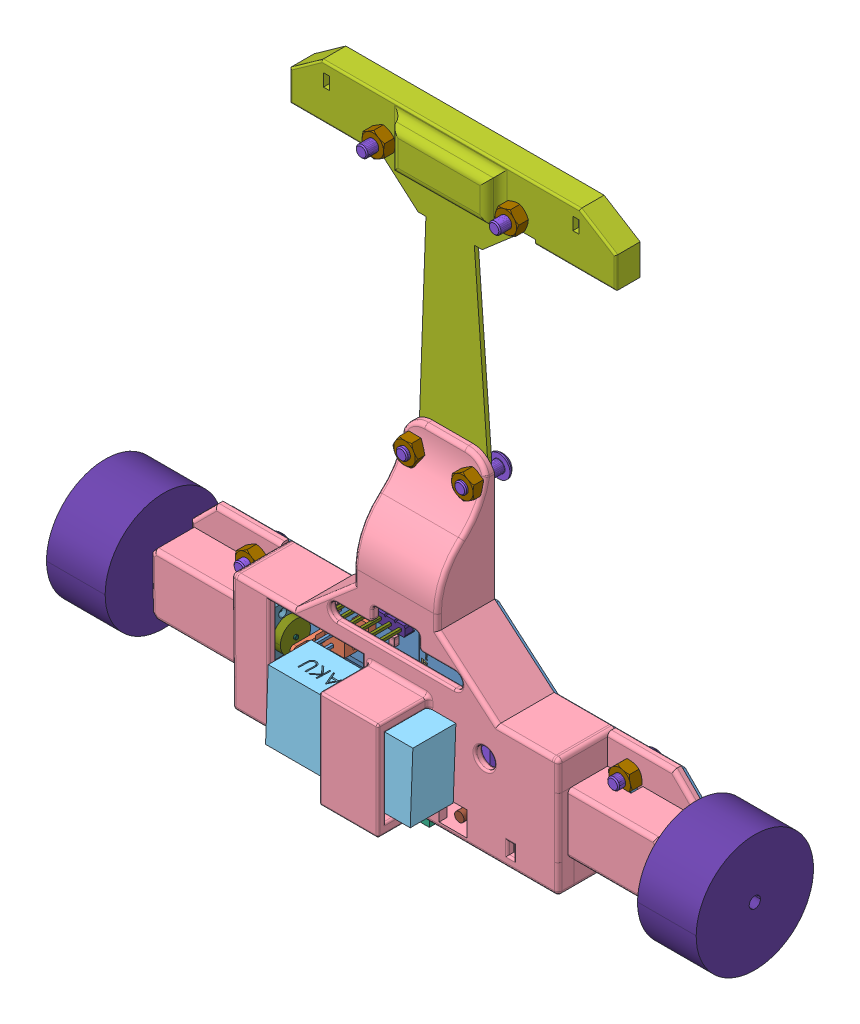
SolidWorks assembly LF_v5_TotalComplexOfRobot, configuration Domyślna. Lengths in mm.
Overall size (166.18 143.38 42.71).
437 component instances, 57 part files, 36 mates.
Components (placement in the parent):
- LF_v5_LowerPartOfHousing-1: LF_v5_LowerPartOfHousing [Domyślna] at (-21.7771 -53.6224 135.3929) size (130 132.75 5.29) (hidden)
- LF_v5_BoardWithSensors.STEP-1: LF_v5_BoardWithSensors.STEP [Domyślna] at (-37.5021 69.0607 133.6929) size (81 20.29 4.87) (hidden)
  - LFEK_Czujniki_v4P_G.step.STEP-1: LFEK_Czujniki_v4P_G.step.STEP [Domyślna] at origin size (81 20.29 4.87)
    - BoardCZV.step.STEP-1: BoardCZV.step.STEP [Domyślna] at origin size (81 20.29 1.59)
      - Open CASCADE STEP translator 6.8 1.1.1.step.STEP-1: Open CASCADE STEP translator 6.8 1.1.1.step.STEP [Domyślna] at (0 0 -1.5914) size (81 20.29 1.59)
    - U8CZV.step.STEP-1: U8CZV.step.STEP [Domyślna] at origin size (4.19 3.05 2)
      - 6801970560.step.STEP-1: 6801970560.step.STEP [Domyślna] at (15.1904 6.573 -3.5914) size (4.19 3.05 2)
        - Extruded.step.STEP-1: Extruded.step.STEP [Domyślna] at origin size (4.19 3.05 2)
    - U7CZV.step.STEP-1: U7CZV.step.STEP [Domyślna] at origin size (4.19 3.05 2)
      - 6801970560.step.STEP-1: 6801970560.step.STEP [Domyślna] at (5.6904 2.473 -3.5914) size (4.19 3.05 2)
        - Extruded.step.STEP-1: Extruded.step.STEP [Domyślna] at origin size (4.19 3.05 2)
    - U6CZV.step.STEP-1: U6CZV.step.STEP [Domyślna] at origin size (4.19 3.05 2)
      - 6801970560.step.STEP-1: 6801970560.step.STEP [Domyślna] at (25.2904 6.673 -3.5914) size (4.19 3.05 2)
        - Extruded.step.STEP-1: Extruded.step.STEP [Domyślna] at origin size (4.19 3.05 2)
    - U5CZV.step.STEP-1: U5CZV.step.STEP [Domyślna] at origin size (4.19 3.05 2)
      - 6801970560.step.STEP-1: 6801970560.step.STEP [Domyślna] at (34.9905 6.673 -3.5914) size (4.19 3.05 2)
        - Extruded.step.STEP-1: Extruded.step.STEP [Domyślna] at origin size (4.19 3.05 2)
    - U4CZV.step.STEP-1: U4CZV.step.STEP [Domyślna] at origin size (4.19 3.05 2)
      - 6801970560.step.STEP-1: 6801970560.step.STEP [Domyślna] at (44.9905 6.673 -3.5914) size (4.19 3.05 2)
        - Extruded.step.STEP-1: Extruded.step.STEP [Domyślna] at origin size (4.19 3.05 2)
    - U3CZV.step.STEP-1: U3CZV.step.STEP [Domyślna] at origin size (4.19 3.05 2)
      - 6801970560.step.STEP-1: 6801970560.step.STEP [Domyślna] at (54.9905 6.673 -3.5914) size (4.19 3.05 2)
        - Extruded.step.STEP-1: Extruded.step.STEP [Domyślna] at origin size (4.19 3.05 2)
    - U2CZV.step.STEP-1: U2CZV.step.STEP [Domyślna] at origin size (4.19 3.05 2)
      - 6801970560.step.STEP-1: 6801970560.step.STEP [Domyślna] at (64.9904 6.673 -3.5914) size (4.19 3.05 2)
        - Extruded.step.STEP-1: Extruded.step.STEP [Domyślna] at origin size (4.19 3.05 2)
    - U1CZV.step.STEP-1: U1CZV.step.STEP [Domyślna] at origin size (4.19 3.05 2)
      - 6801970560.step.STEP-1: 6801970560.step.STEP [Domyślna] at (74.7905 2.373 -3.5914) size (4.19 3.05 2)
        - Extruded.step.STEP-1: Extruded.step.STEP [Domyślna] at origin size (4.19 3.05 2)
    - D2CZV.step.STEP-1: D2CZV.step.STEP [Domyślna] at origin size (1.6 3.2 1.1)
      - D1206_2.step.STEP-1: D1206_2.step.STEP [Domyślna] at (8.2001 8.2337 0.2489) x (0 1 0) z (1 0 0) size (3.2 1.1 1.6)
    - D1CZV.step.STEP-1: D1CZV.step.STEP [Domyślna] at origin size (1.6 3.2 1.1)
      - D1206_2.step.STEP-1: D1206_2.step.STEP [Domyślna] at (71.9999 8.3333 0.2489) x (0 -1 0) z (-1 0 0) size (3.2 1.1 1.6)
    - J1CZV.step.STEP-1: J1CZV.step.STEP [Domyślna] at origin size (15.7 4.25 1.29)
      - 687120183722.step.STEP-1: 687120183722.step.STEP [Domyślna] at (39.9501 4.8501 0.64) x (1 0 0) z (0 0 1) size (15.7 4.25 1.29)
        - 68x120183x22.step.STEP-1: 68x120183x22.step.STEP [Domyślna] at origin size (13 3.1 1.2)
        - 68X1xx183x22_Pin_Bottom.step.STEP-1: 68X1xx183x22_Pin_Bottom.step.STEP [Domyślna] at (-4.65 1.05 0.005) x (0 1 0) z (0 0 1) size (3.1 0.2 1.15)
        - 68x120183x22_Actuator.step.STEP-1: 68x120183x22_Actuator.step.STEP [Domyślna] at (0 -2 0) x (1 0 0) z (0 0 -1) size (15.7 3.8 1.1)
        - 68X1XX183X22_Solder_Pad.step.STEP-1: 68X1XX183X22_Solder_Pad.step.STEP [Domyślna] at (5.55 -0.25 0.02) x (0 -1 0) z (0 0 1) size (2.5 2 1.24)
        - 68X1xx183x22_Solder_Pad2.step.STEP-1: 68X1xx183x22_Solder_Pad2.step.STEP [Domyślna] at (-5.55 -0.25 0.02) x (0 -1 0) z (0 0 -1) size (2.5 2 1.24)
        - 68X1xx183x22_Pin_Bottom.step.STEP-2: 68X1xx183x22_Pin_Bottom.step.STEP [Domyślna] at (-4.15 1.05 0.005) x (0 1 0) z (0 0 1) size (3.1 0.2 1.15)
        - 68X1xx183x22_Pin_Bottom.step.STEP-3: 68X1xx183x22_Pin_Bottom.step.STEP [Domyślna] at (-3.65 1.05 0.005) x (0 1 0) z (0 0 1) size (3.1 0.2 1.15)
        - 68X1xx183x22_Pin_Bottom.step.STEP-4: 68X1xx183x22_Pin_Bottom.step.STEP [Domyślna] at (-3.15 1.05 0.005) x (0 1 0) z (0 0 1) size (3.1 0.2 1.15)
        - 68X1xx183x22_Pin_Bottom.step.STEP-5: 68X1xx183x22_Pin_Bottom.step.STEP [Domyślna] at (-2.65 1.05 0.005) x (0 1 0) z (0 0 1) size (3.1 0.2 1.15)
        - 68X1xx183x22_Pin_Bottom.step.STEP-6: 68X1xx183x22_Pin_Bottom.step.STEP [Domyślna] at (-2.15 1.05 0.005) x (0 1 0) z (0 0 1) size (3.1 0.2 1.15)
        - 68X1xx183x22_Pin_Bottom.step.STEP-7: 68X1xx183x22_Pin_Bottom.step.STEP [Domyślna] at (-1.65 1.05 0.005) x (0 1 0) z (0 0 1) size (3.1 0.2 1.15)
        - 68X1xx183x22_Pin_Bottom.step.STEP-8: 68X1xx183x22_Pin_Bottom.step.STEP [Domyślna] at (-1.15 1.05 0.005) x (0 1 0) z (0 0 1) size (3.1 0.2 1.15)
        - 68X1xx183x22_Pin_Bottom.step.STEP-9: 68X1xx183x22_Pin_Bottom.step.STEP [Domyślna] at (-0.65 1.05 0.005) x (0 1 0) z (0 0 1) size (3.1 0.2 1.15)
        - 68X1xx183x22_Pin_Bottom.step.STEP-10: 68X1xx183x22_Pin_Bottom.step.STEP [Domyślna] at (-0.15 1.05 0.005) x (0 1 0) z (0 0 1) size (3.1 0.2 1.15)
        - 68X1xx183x22_Pin_Bottom.step.STEP-11: 68X1xx183x22_Pin_Bottom.step.STEP [Domyślna] at (0.35 1.05 0.005) x (0 1 0) z (0 0 1) size (3.1 0.2 1.15)
        - 68X1xx183x22_Pin_Bottom.step.STEP-12: 68X1xx183x22_Pin_Bottom.step.STEP [Domyślna] at (0.85 1.05 0.005) x (0 1 0) z (0 0 1) size (3.1 0.2 1.15)
        - 68X1xx183x22_Pin_Bottom.step.STEP-13: 68X1xx183x22_Pin_Bottom.step.STEP [Domyślna] at (1.35 1.05 0.005) x (0 1 0) z (0 0 1) size (3.1 0.2 1.15)
        - 68X1xx183x22_Pin_Bottom.step.STEP-14: 68X1xx183x22_Pin_Bottom.step.STEP [Domyślna] at (1.85 1.05 0.005) x (0 1 0) z (0 0 1) size (3.1 0.2 1.15)
        - 68X1xx183x22_Pin_Bottom.step.STEP-15: 68X1xx183x22_Pin_Bottom.step.STEP [Domyślna] at (2.35 1.05 0.005) x (0 1 0) z (0 0 1) size (3.1 0.2 1.15)
        - 68X1xx183x22_Pin_Bottom.step.STEP-16: 68X1xx183x22_Pin_Bottom.step.STEP [Domyślna] at (2.85 1.05 0.005) x (0 1 0) z (0 0 1) size (3.1 0.2 1.15)
        - 68X1xx183x22_Pin_Bottom.step.STEP-17: 68X1xx183x22_Pin_Bottom.step.STEP [Domyślna] at (3.35 1.05 0.005) x (0 1 0) z (0 0 1) size (3.1 0.2 1.15)
        - 68X1xx183x22_Pin_Bottom.step.STEP-18: 68X1xx183x22_Pin_Bottom.step.STEP [Domyślna] at (3.85 1.05 0.005) x (0 1 0) z (0 0 1) size (3.1 0.2 1.15)
        - 68X1xx183x22_Pin_Bottom.step.STEP-19: 68X1xx183x22_Pin_Bottom.step.STEP [Domyślna] at (4.35 1.05 0.005) x (0 1 0) z (0 0 1) size (3.1 0.2 1.15)
        - 68X1xx183x22_Pin_Bottom.step.STEP-20: 68X1xx183x22_Pin_Bottom.step.STEP [Domyślna] at (4.85 1.05 0.005) x (0 1 0) z (0 0 1) size (3.1 0.2 1.15)
    - R1CZV.step.STEP-1: R1CZV.step.STEP [Domyślna] at origin size (1.25 2 0.6)
      - User_Library-SMD_RESISTOR-10805.step.STEP-1: User_Library-SMD_RESISTOR-10805.step.STEP [Domyślna] at (78.94 2.4538 -1.881) x (1 0 0) z (0 -1 0) size (1.25 0.6 2)
    - R2CZV.step.STEP-1: R2CZV.step.STEP [Domyślna] at origin size (1.25 2 0.6)
      - User_Library-SMD_RESISTOR-10805.step.STEP-1: User_Library-SMD_RESISTOR-10805.step.STEP [Domyślna] at (59.1239 6.7758 -1.881) x (1 0 0) z (0 -1 0) size (1.25 0.6 2)
    - R3CZV.step.STEP-1: R3CZV.step.STEP [Domyślna] at origin size (1.25 2 0.6)
      - User_Library-SMD_RESISTOR-10805.step.STEP-1: User_Library-SMD_RESISTOR-10805.step.STEP [Domyślna] at (48.7205 6.6898 -1.881) x (1 0 0) z (0 -1 0) size (1.25 0.6 2)
    - R4CZV.step.STEP-1: R4CZV.step.STEP [Domyślna] at origin size (1.25 2 0.6)
      - User_Library-SMD_RESISTOR-10805.step.STEP-1: User_Library-SMD_RESISTOR-10805.step.STEP [Domyślna] at (68.9209 6.8237 -1.881) x (1 0 0) z (0 -1 0) size (1.25 0.6 2)
    - R5CZV.step.STEP-1: R5CZV.step.STEP [Domyślna] at origin size (2 1.25 0.6)
      - User_Library-SMD_RESISTOR-10805.step.STEP-1: User_Library-SMD_RESISTOR-10805.step.STEP [Domyślna] at (69.9592 3.2749 -1.881) x (0 1 0) z (1 0 0) size (1.25 0.6 2)
    - R6CZV.step.STEP-1: R6CZV.step.STEP [Domyślna] at origin size (1.25 2 0.6)
      - User_Library-SMD_RESISTOR-10805.step.STEP-1: User_Library-SMD_RESISTOR-10805.step.STEP [Domyślna] at (50.6149 6.6488 -1.881) x (1 0 0) z (0 -1 0) size (1.25 0.6 2)
    - R7CZV.step.STEP-1: R7CZV.step.STEP [Domyślna] at origin size (2 1.25 0.6)
      - User_Library-SMD_RESISTOR-10805.step.STEP-1: User_Library-SMD_RESISTOR-10805.step.STEP [Domyślna] at (45.1658 9.5901 -1.881) x (0 -1 0) z (-1 0 0) size (1.25 0.6 2)
    - R8CZV.step.STEP-1: R8CZV.step.STEP [Domyślna] at origin size (1.25 2 0.6)
      - User_Library-SMD_RESISTOR-10805.step.STEP-1: User_Library-SMD_RESISTOR-10805.step.STEP [Domyślna] at (61.1499 6.7158 -1.881) x (1 0 0) z (0 -1 0) size (1.25 0.6 2)
    - R9CZV.step.STEP-1: R9CZV.step.STEP [Domyślna] at origin size (2 1.25 0.6)
      - User_Library-SMD_RESISTOR-10805.step.STEP-1: User_Library-SMD_RESISTOR-10805.step.STEP [Domyślna] at (34.7912 9.608 -1.881) x (0 1 0) z (1 0 0) size (1.25 0.6 2)
    - R10CZV.step.STEP-1: R10CZV.step.STEP [Domyślna] at origin size (1.25 2 0.6)
      - User_Library-SMD_RESISTOR-10805.step.STEP-1: User_Library-SMD_RESISTOR-10805.step.STEP [Domyślna] at (29.0439 6.7928 -1.881) x (1 0 0) z (0 -1 0) size (1.25 0.6 2)
    - R11CZV.step.STEP-1: R11CZV.step.STEP [Domyślna] at origin size (2 1.25 0.6)
      - User_Library-SMD_RESISTOR-10805.step.STEP-1: User_Library-SMD_RESISTOR-10805.step.STEP [Domyślna] at (7.9162 5.5999 -1.881) x (0 1 0) z (1 0 0) size (1.25 0.6 2)
    - R12CZV.step.STEP-1: R12CZV.step.STEP [Domyślna] at origin size (1.25 2 0.6)
      - User_Library-SMD_RESISTOR-10805.step.STEP-1: User_Library-SMD_RESISTOR-10805.step.STEP [Domyślna] at (19.1249 6.6337 -1.881) x (1 0 0) z (0 -1 0) size (1.25 0.6 2)
    - R13CZV.step.STEP-1: R13CZV.step.STEP [Domyślna] at origin size (1.25 2 0.6)
      - User_Library-SMD_RESISTOR-10805.step.STEP-1: User_Library-SMD_RESISTOR-10805.step.STEP [Domyślna] at (31.0839 6.9058 -1.881) x (1 0 0) z (0 -1 0) size (1.25 0.6 2)
    - R14CZV.step.STEP-1: R14CZV.step.STEP [Domyślna] at origin size (1.25 2 0.6)
      - User_Library-SMD_RESISTOR-10805.step.STEP-1: User_Library-SMD_RESISTOR-10805.step.STEP [Domyślna] at (21.3409 6.6698 -1.881) x (1 0 0) z (0 -1 0) size (1.25 0.6 2)
    - R15CZV.step.STEP-1: R15CZV.step.STEP [Domyślna] at origin size (1.25 2 0.6)
      - User_Library-SMD_RESISTOR-10805.step.STEP-1: User_Library-SMD_RESISTOR-10805.step.STEP [Domyślna] at (11.3899 6.7318 -1.881) x (1 0 0) z (0 -1 0) size (1.25 0.6 2)
    - R16CZV.step.STEP-1: R16CZV.step.STEP [Domyślna] at origin size (1.25 2 0.6)
      - User_Library-SMD_RESISTOR-10805.step.STEP-1: User_Library-SMD_RESISTOR-10805.step.STEP [Domyślna] at (1.6869 2.2537 -1.881) x (1 0 0) z (0 -1 0) size (1.25 0.6 2)
- LF_v5_MainElectricalBoardwithMCU.step-1: LF_v5_MainElectricalBoardwithMCU.step [Domyślna] at (-21.7771 -53.6224 135.3929) size (166.18 41.84 30.14)
  - BoardFF.step-1: BoardFF.step [Domyślna] at origin size (130 40.35 1.59)
    - Open CASCADE STEP translator 6.8 2.1.1.step-1: Open CASCADE STEP translator 6.8 2.1.1.step [Domyślna] at (0 0 -1.5914) size (130 40.35 1.59)
  - CMJ1FF.step-1: CMJ1FF.step [Domyślna] at origin size (4.19 3.05 2)
    - 6480266160.step-1: 6480266160.step [Domyślna] at (3.27 16.79 0) size (4.19 3.05 2)
      - Extruded.step-1: Extruded.step [Domyślna] at origin size (4.19 3.05 2)
  - CMJ2FF.step-1: CMJ2FF.step [Domyślna] at origin size (8.61 4.54 5)
    - 6480265920.step-1: 6480265920.step [Domyślna] at (47.73 6.385 0) size (8.61 4.54 5)
      - Extruded-0.step-1: Extruded-0.step [Domyślna] at origin size (8.61 4.54 5)
  - C4FF.step-1: C4FF.step [Domyślna] at origin size (1.35 2.1 1.35)
    - 0805C.step-1: 0805C.step [Domyślna] at (54.4661 6.0661 0) x (0 -1 0) z (0 0 1) size (2.1 1.35 1.35)
      - Open CASCADE STEP translator 6.8 2.4.1.1.step-1: Open CASCADE STEP translator 6.8 2.4.1.1.step [Domyślna] at origin size (2.1 1.35 1.35)
      - Open CASCADE STEP translator 6.8 2.4.1.2.step-1: Open CASCADE STEP translator 6.8 2.4.1.2.step [Domyślna] at origin
  - U6FF.step-1: U6FF.step [Domyślna] at origin size (7 6.5 1.65)
    - SOT-223.step-1: SOT-223.step [Domyślna] at (3.0406 1.7749 -2.3167) x (-1 0 0) z (0 -1 0) size (7 1.65 6.5)
  - 16FF.step-1: 16FF.step [Domyślna] at origin size (3.39 1.6 1.65)
    - 3216-SMDA.step-1: 3216-SMDA.step [Domyślna] at (47.0511 -1.8714 -0.4115) x (1 0 0) z (0 0 1) size (3.39 1.6 1.65)
      - User_Library-Tantalum_Capacitor_Case_A_Tantalum_case_A_part1.step-1: User_Library-Tantalum_Capacitor_Case_A_Tantalum_case_A_part1.step [Domyślna] at (-1.4503 0.3155 0.551) size (3.2 1.6 1.6)
      - User_Library-Tantalum_Capacitor_Case_A_Tantalum_case_A_part2.step-1: User_Library-Tantalum_Capacitor_Case_A_Tantalum_case_A_part2.step [Domyślna] at (-0.7455 0.5155 0.501) x (-1 0 0) z (0 0 -1) size (0.8 1.2 0.9)
      - User_Library-Tantalum_Capacitor_Case_A_Tantalum_case_A_part2.step-2: User_Library-Tantalum_Capacitor_Case_A_Tantalum_case_A_part2.step [Domyślna] at (1.0449 1.7155 0.501) x (1 0 0) z (0 0 -1) size (0.8 1.2 0.9)
  - D4FF.step-1: D4FF.step [Domyślna] at origin size (6.11 8.13 2.39)
    - DO214AB.step-1: DO214AB.step [Domyślna] at (-8.5231 8.9094 -1.566) x (0 1 0) z (0 0 -1) size (8.13 6.11 2.39)
  - P3FF.step-1: P3FF.step [Domyślna] at origin size (2.54 10.16 11.54)
    - 61300411121.step-1: 61300411121.step [Domyślna] at (13.85 2.18 1.3) x (0 1 0) z (1 0 0) size (10.16 11.54 2.54)
      - 6130xx11121_PIN.step-1: 6130xx11121_PIN.step [Domyślna] at (-3.81 1.5 0) x (1 0 0) z (0 -1 0) size (0.64 0.64 11.54)
      - 6130xx11121_PIN.step-2: 6130xx11121_PIN.step [Domyślna] at (-1.27 1.5 0) x (1 0 0) z (0 -1 0) size (0.64 0.64 11.54)
      - 6130xx11121_PIN.step-3: 6130xx11121_PIN.step [Domyślna] at (1.27 1.5 0) x (1 0 0) z (0 -1 0) size (0.64 0.64 11.54)
      - 6130xx11121_PIN.step-4: 6130xx11121_PIN.step [Domyślna] at (3.81 1.5 0) x (1 0 0) z (0 -1 0) size (0.64 0.64 11.54)
      - 61300411121-1.step-1: 61300411121-1.step [Domyślna] at origin size (10.16 2.54 2.54)
  - IR_TSOP2236FF.step-1: IR_TSOP2236FF.step [Domyślna] at origin size (2.4 2.4 13)
    - 6479903328.step-1: 6479903328.step [Domyślna] at (39.625 -1.7875 0) x (-1 0 0) z (0 0 1) size (2.4 2.4 13)
      - Cylinder.step-1: Cylinder.step [Domyślna] at origin size (2.4 2.4 13)
  - R10FF.step-1: R10FF.step [Domyślna] at origin size (2 1.25 0.6)
    - User_Library-SMD_RESISTOR-10805.step-1: User_Library-SMD_RESISTOR-10805.step [Domyślna] at (14.3657 29.675 0.2896) x (0 -1 0) z (-1 0 0) size (1.25 0.6 2)
  - R9FF.step-1: R9FF.step [Domyślna] at origin size (2 1.25 0.6)
    - User_Library-SMD_RESISTOR-10805.step-1: User_Library-SMD_RESISTOR-10805.step [Domyślna] at (14.3907 31.6001 0.2896) x (0 -1 0) z (-1 0 0) size (1.25 0.6 2)
  - C25FF.step-1: C25FF.step [Domyślna] at origin size (1.35 2.1 1.35)
    - 0805C.step-1: 0805C.step [Domyślna] at (43.9001 15.4161 0) x (0 -1 0) z (0 0 1) size (2.1 1.35 1.35)
      - Open CASCADE STEP translator 6.8 2.4.1.1.step-1: Open CASCADE STEP translator 6.8 2.4.1.1.step [Domyślna] at origin size (2.1 1.35 1.35)
      - Open CASCADE STEP translator 6.8 2.4.1.2.step-1: Open CASCADE STEP translator 6.8 2.4.1.2.step [Domyślna] at origin
  - C30FF.step-1: C30FF.step [Domyślna] at origin size (1.35 2.1 1.35)
    - 0805C.step-1: 0805C.step [Domyślna] at (43.8749 17.3089 0) x (0 1 0) z (0 0 1) size (2.1 1.35 1.35)
      - Open CASCADE STEP translator 6.8 2.4.1.1.step-1: Open CASCADE STEP translator 6.8 2.4.1.1.step [Domyślna] at origin size (2.1 1.35 1.35)
      - Open CASCADE STEP translator 6.8 2.4.1.2.step-1: Open CASCADE STEP translator 6.8 2.4.1.2.step [Domyślna] at origin
  - C28FF.step-1: C28FF.step [Domyślna] at origin size (1.71 3.2 1.71)
    - User_Library-Capacitor_Vishay_1206_X7R.step-1: User_Library-Capacitor_Vishay_1206_X7R.step [Domyślna] at (14.9319 10.1506 -0.0102) x (0 1 0) z (0 0 1) size (3.2 1.7 1.7)
  - R14FF.step-1: R14FF.step [Domyślna] at origin size (1.25 2 0.6)
    - User_Library-SMD_RESISTOR-10805.step-1: User_Library-SMD_RESISTOR-10805.step [Domyślna] at (41.1749 1.7657 0.2896) x (1 0 0) z (0 -1 0) size (1.25 0.6 2)
  - R13FF.step-1: R13FF.step [Domyślna] at origin size (2 1.25 0.6)
    - User_Library-SMD_RESISTOR-10805.step-1: User_Library-SMD_RESISTOR-10805.step [Domyślna] at (37.4236 9.82 0.2896) x (0 -1 0) z (-1 0 0) size (1.25 0.6 2)
  - U2FF.step-1: U2FF.step [Domyślna] at origin size (49.09 30.14 30.14)
    - Silnik_enkAP214.step-1: Silnik_enkAP214.step [Domyślna] at (64.0421 1.0451 0) x (0 0 -1) z (0 1 0) size (30.14 49.09 30.14)
      - Enkoder_PCB.step-1: Enkoder_PCB.step [Domyślna] at (-5.6332 0.2835 8.6889) x (0 0 1) z (0 1 0) size (11.6 9.6 1.3)
      - micro-metal-gearmotor-backshaft.step.step-1: micro-metal-gearmotor-backshaft.step.step [Domyślna] at (-5.6332 -15.9165 8.6889) x (0 0 1) z (0 -1 0) size (12 10.04 40.2)
      - Dysk_pololu.step-1: Dysk_pololu.step [Domyślna] at (-5.6332 -14.4184 8.6889) x (0.89461 0 0.446849) z (0 1 0) size (7.7 7.7 2)
      - Dysk_pololu.step-2: Dysk_pololu.step [Domyślna] at (-5.6332 4.8635 8.6889) x (0.999981 0 -0.006181) z (0 -1 0) size (7.7 7.7 2)
      - Kolko.step-1: Kolko.step [Domyślna] at (-5.6332 -28.8098 8.6889) x (0.999989 0 -0.004766) z (0 -1 0) size (30 30 15)
  - U1FF.step-1: U1FF.step [Domyślna] at origin size (49.09 30.14 30.14)
    - Silnik_enkAP214.step-1: Silnik_enkAP214.step [Domyślna] at (-14.5171 18.505 0) x (0 0 -1) z (0 -1 0) size (30.14 49.09 30.14)
      - Enkoder_PCB.step-1: Enkoder_PCB.step [Domyślna] at (-5.6332 0.2835 8.6889) x (0 0 1) z (0 1 0) size (11.6 9.6 1.3)
      - micro-metal-gearmotor-backshaft.step.step-1: micro-metal-gearmotor-backshaft.step.step [Domyślna] at (-5.6332 -15.9165 8.6889) x (0 0 1) z (0 -1 0) size (12 10.04 40.2)
      - Dysk_pololu.step-1: Dysk_pololu.step [Domyślna] at (-5.6332 -14.4184 8.6889) x (0.89461 0 0.446849) z (0 1 0) size (7.7 7.7 2)
      - Dysk_pololu.step-2: Dysk_pololu.step [Domyślna] at (-5.6332 4.8635 8.6889) x (0.999981 0 -0.006181) z (0 -1 0) size (7.7 7.7 2)
      - Kolko.step-1: Kolko.step [Domyślna] at (-5.6332 -28.8098 8.6889) x (0.999989 0 -0.004766) z (0 -1 0) size (30 30 15)
  - Y1FF.step-1: Y1FF.step [Domyślna] at origin size (3.27 5.5 1.5)
    - 6479903888.step-1: 6479903888.step [Domyślna] at (41.0546 16.3547 0) size (3.27 5.5 1.5)
      - Extruded-2.step-1: Extruded-2.step [Domyślna] at origin size (3.27 5.5 1.5)
  - VIN_CONNECTOR1FF.step-1: VIN_CONNECTOR1FF.step [Domyślna] at origin size (5.8 5.08 14.9)
    - 61900211121.step-1: 61900211121.step [Domyślna] at (-2.2999 11.5249 5.78) x (0 1 0) z (0 0 1) size (5.08 5.8 14.9)
      - 6190xx11121_PIN.step-1: 6190xx11121_PIN.step [Domyślna] at (-1.27 0.3 -2.05) size (0.64 0.64 14.2)
      - 6190xx11121_PIN.step-2: 6190xx11121_PIN.step [Domyślna] at (1.27 0.3 -1.75) size (0.64 0.64 14.2)
      - 61900211121-3.step-1: 61900211121-3.step [Domyślna] at origin size (5.08 5.8 11.5)
  - U4FF.step-1: U4FF.step [Domyślna] at origin size (6.42 5 1)
    - PW0016AakaMTC16.step-1: PW0016AakaMTC16.step [Domyślna] at (47.7419 6.5511 -2.1914) x (0 -1 0) z (1 0 0) size (5 1 6.42)
      - BODY_MTC16.step-1: BODY_MTC16.step [Domyślna] at origin size (5 0.9 4.4)
      - LEAD_MTC16.step-1: LEAD_MTC16.step [Domyślna] at (2.275 -0.3725 -2.6) x (-1 0 0) z (0 0 -1) size (0.24 0.62 1.01)
      - LEAD_MTC16.step-2: LEAD_MTC16.step [Domyślna] at (1.625 -0.3725 -2.6) x (-1 0 0) z (0 0 -1) size (0.24 0.62 1.01)
      - LEAD_MTC16.step-3: LEAD_MTC16.step [Domyślna] at (0.975 -0.3725 -2.6) x (-1 0 0) z (0 0 -1) size (0.24 0.62 1.01)
      - LEAD_MTC16.step-4: LEAD_MTC16.step [Domyślna] at (0.325 -0.3725 -2.6) x (-1 0 0) z (0 0 -1) size (0.24 0.62 1.01)
      - LEAD_MTC16.step-5: LEAD_MTC16.step [Domyślna] at (-0.325 -0.3725 -2.6) x (-1 0 0) z (0 0 -1) size (0.24 0.62 1.01)
      - LEAD_MTC16.step-6: LEAD_MTC16.step [Domyślna] at (-0.975 -0.3725 -2.6) x (-1 0 0) z (0 0 -1) size (0.24 0.62 1.01)
      - LEAD_MTC16.step-7: LEAD_MTC16.step [Domyślna] at (-1.625 -0.3725 -2.6) x (-1 0 0) z (0 0 -1) size (0.24 0.62 1.01)
      - LEAD_MTC16.step-8: LEAD_MTC16.step [Domyślna] at (-2.275 -0.3725 -2.6) x (-1 0 0) z (0 0 -1) size (0.24 0.62 1.01)
      - LEAD_MTC16.step-9: LEAD_MTC16.step [Domyślna] at (2.275 -0.3725 2.6) size (0.24 0.62 1.01)
      - LEAD_MTC16.step-10: LEAD_MTC16.step [Domyślna] at (1.625 -0.3725 2.6) size (0.24 0.62 1.01)
      - LEAD_MTC16.step-11: LEAD_MTC16.step [Domyślna] at (0.975 -0.3725 2.6) size (0.24 0.62 1.01)
      - LEAD_MTC16.step-12: LEAD_MTC16.step [Domyślna] at (0.325 -0.3725 2.6) size (0.24 0.62 1.01)
      - LEAD_MTC16.step-13: LEAD_MTC16.step [Domyślna] at (-0.325 -0.3725 2.6) size (0.24 0.62 1.01)
      - LEAD_MTC16.step-14: LEAD_MTC16.step [Domyślna] at (-0.975 -0.3725 2.6) size (0.24 0.62 1.01)
      - LEAD_MTC16.step-15: LEAD_MTC16.step [Domyślna] at (-1.625 -0.3725 2.6) size (0.24 0.62 1.01)
      - LEAD_MTC16.step-16: LEAD_MTC16.step [Domyślna] at (-2.275 -0.3725 2.6) size (0.24 0.62 1.01)
  - U3FF.step-1: U3FF.step [Domyślna] at origin size (6.42 5 1)
    - PW0016AakaMTC16.step-1: PW0016AakaMTC16.step [Domyślna] at (3.035 17.0029 -2.1914) x (0 1 0) z (-1 0 0) size (5 1 6.42)
      - BODY_MTC16.step-1: BODY_MTC16.step [Domyślna] at origin size (5 0.9 4.4)
      - LEAD_MTC16.step-1: LEAD_MTC16.step [Domyślna] at (2.275 -0.3725 -2.6) x (-1 0 0) z (0 0 -1) size (0.24 0.62 1.01)
      - LEAD_MTC16.step-2: LEAD_MTC16.step [Domyślna] at (1.625 -0.3725 -2.6) x (-1 0 0) z (0 0 -1) size (0.24 0.62 1.01)
      - LEAD_MTC16.step-3: LEAD_MTC16.step [Domyślna] at (0.975 -0.3725 -2.6) x (-1 0 0) z (0 0 -1) size (0.24 0.62 1.01)
      - LEAD_MTC16.step-4: LEAD_MTC16.step [Domyślna] at (0.325 -0.3725 -2.6) x (-1 0 0) z (0 0 -1) size (0.24 0.62 1.01)
      - LEAD_MTC16.step-5: LEAD_MTC16.step [Domyślna] at (-0.325 -0.3725 -2.6) x (-1 0 0) z (0 0 -1) size (0.24 0.62 1.01)
      - LEAD_MTC16.step-6: LEAD_MTC16.step [Domyślna] at (-0.975 -0.3725 -2.6) x (-1 0 0) z (0 0 -1) size (0.24 0.62 1.01)
      - LEAD_MTC16.step-7: LEAD_MTC16.step [Domyślna] at (-1.625 -0.3725 -2.6) x (-1 0 0) z (0 0 -1) size (0.24 0.62 1.01)
      - LEAD_MTC16.step-8: LEAD_MTC16.step [Domyślna] at (-2.275 -0.3725 -2.6) x (-1 0 0) z (0 0 -1) size (0.24 0.62 1.01)
      - LEAD_MTC16.step-9: LEAD_MTC16.step [Domyślna] at (2.275 -0.3725 2.6) size (0.24 0.62 1.01)
      - LEAD_MTC16.step-10: LEAD_MTC16.step [Domyślna] at (1.625 -0.3725 2.6) size (0.24 0.62 1.01)
      - LEAD_MTC16.step-11: LEAD_MTC16.step [Domyślna] at (0.975 -0.3725 2.6) size (0.24 0.62 1.01)
      - LEAD_MTC16.step-12: LEAD_MTC16.step [Domyślna] at (0.325 -0.3725 2.6) size (0.24 0.62 1.01)
      - LEAD_MTC16.step-13: LEAD_MTC16.step [Domyślna] at (-0.325 -0.3725 2.6) size (0.24 0.62 1.01)
      - LEAD_MTC16.step-14: LEAD_MTC16.step [Domyślna] at (-0.975 -0.3725 2.6) size (0.24 0.62 1.01)
      - LEAD_MTC16.step-15: LEAD_MTC16.step [Domyślna] at (-1.625 -0.3725 2.6) size (0.24 0.62 1.01)
      - LEAD_MTC16.step-16: LEAD_MTC16.step [Domyślna] at (-2.275 -0.3725 2.6) size (0.24 0.62 1.01)
  - S1FF.step-1: S1FF.step [Domyślna] at origin size (5.3 6.4 1.4)
    - User_Library-button1.step-1: User_Library-button1.step [Domyślna] at (47.7484 16.0669 0) x (0 1 0) z (1 0 0) size (6.4 1.4 5.3)
  - R27FF.step-1: R27FF.step [Domyślna] at origin size (1.6 3.2 0.6)
    - User_Library-SMD_RESISTOR-11206.step-1: User_Library-SMD_RESISTOR-11206.step [Domyślna] at (38.225 17.9491 0.3048) x (1 0 0) z (0 -1 0) size (1.6 0.6 3.2)
  - R21FF.step-1: R21FF.step [Domyślna] at origin size (1.6 3.2 0.6)
    - User_Library-SMD_RESISTOR-11206.step-1: User_Library-SMD_RESISTOR-11206.step [Domyślna] at (53.6035 17.591 0.3048) x (1 0 0) z (0 -1 0) size (1.6 0.6 3.2)
  - R20FF.step-1: R20FF.step [Domyślna] at origin size (1.6 3.2 0.6)
    - User_Library-SMD_RESISTOR-11206.step-1: User_Library-SMD_RESISTOR-11206.step [Domyślna] at (34.0249 -1.0387 0.3048) x (1 0 0) z (0 -1 0) size (1.6 0.6 3.2)
  - R19FF.step-1: R19FF.step [Domyślna] at origin size (1.25 2 0.6)
    - User_Library-SMD_RESISTOR-10805.step-1: User_Library-SMD_RESISTOR-10805.step [Domyślna] at (8.4895 11.0588 0.2896) x (1 0 0) z (0 -1 0) size (1.25 0.6 2)
  - R18FF.step-1: R18FF.step [Domyślna] at origin size (1.25 2 0.6)
    - User_Library-SMD_RESISTOR-10805.step-1: User_Library-SMD_RESISTOR-10805.step [Domyślna] at (10.3694 11.0908 0.2896) x (1 0 0) z (0 -1 0) size (1.25 0.6 2)
  - R17FF.step-1: R17FF.step [Domyślna] at origin size (1.25 2 0.6)
    - User_Library-SMD_RESISTOR-10805.step-1: User_Library-SMD_RESISTOR-10805.step [Domyślna] at (2.85 11.0088 0.2896) x (1 0 0) z (0 -1 0) size (1.25 0.6 2)
  - R16FF.step-1: R16FF.step [Domyślna] at origin size (1.25 2 0.6)
    - User_Library-SMD_RESISTOR-10805.step-1: User_Library-SMD_RESISTOR-10805.step [Domyślna] at (4.7297 11.0088 0.2896) x (1 0 0) z (0 -1 0) size (1.25 0.6 2)
  - R15FF.step-1: R15FF.step [Domyślna] at origin size (1.25 2 0.6)
    - User_Library-SMD_RESISTOR-10805.step-1: User_Library-SMD_RESISTOR-10805.step [Domyślna] at (6.6096 11.0088 0.2896) x (1 0 0) z (0 -1 0) size (1.25 0.6 2)
  - R12FF.step-1: R12FF.step [Domyślna] at origin size (1.6 3.2 0.6)
    - User_Library-SMD_RESISTOR-11206.step-1: User_Library-SMD_RESISTOR-11206.step [Domyślna] at (10.3339 26.076 0.3048) x (-1 0 0) z (0 1 0) size (1.6 0.6 3.2)
  - R8FF.step-1: R8FF.step [Domyślna] at origin size (3.2 1.6 0.6)
    - User_Library-SMD_RESISTOR-11206.step-1: User_Library-SMD_RESISTOR-11206.step [Domyślna] at (47.3989 2.275 0.3048) x (0 1 0) z (1 0 0) size (1.6 0.6 3.2)
  - R7FF.step-1: R7FF.step [Domyślna] at origin size (1.6 0.8 0.45)
    - User_Library-SMD_RESISTOR-10603.step-1: User_Library-SMD_RESISTOR-10603.step [Domyślna] at (4.7379 19.45 0.2159) x (0 -1 0) z (-1 0 0) size (0.8 0.45 1.6)
  - R6FF.step-1: R6FF.step [Domyślna] at origin size (3.2 1.6 0.6)
    - User_Library-SMD_RESISTOR-11206.step-1: User_Library-SMD_RESISTOR-11206.step [Domyślna] at (56.9509 5.55 -1.8962) x (0 -1 0) z (1 0 0) size (1.6 0.6 3.2)
  - R5FF.step-1: R5FF.step [Domyślna] at origin size (3.2 1.6 0.6)
    - User_Library-SMD_RESISTOR-11206.step-1: User_Library-SMD_RESISTOR-11206.step [Domyślna] at (-6.0239 18.2249 -1.8962) x (0 1 0) z (-1 0 0) size (1.6 0.6 3.2)
  - R4FF.step-1: R4FF.step [Domyślna] at origin size (3.2 1.6 0.6)
    - User_Library-SMD_RESISTOR-11206.step-1: User_Library-SMD_RESISTOR-11206.step [Domyślna] at (57.0239 7.6839 -1.8962) x (0 -1 0) z (1 0 0) size (1.6 0.6 3.2)
  - R3FF.step-1: R3FF.step [Domyślna] at origin size (3.2 1.6 0.6)
    - User_Library-SMD_RESISTOR-11206.step-1: User_Library-SMD_RESISTOR-11206.step [Domyślna] at (47.526 10.5749 0.3048) x (0 1 0) z (1 0 0) size (1.6 0.6 3.2)
  - R1FF.step-1: R1FF.step [Domyślna] at origin size (3.2 1.6 0.6)
    - User_Library-SMD_RESISTOR-11206.step-1: User_Library-SMD_RESISTOR-11206.step [Domyślna] at (-6.074 16.0912 -1.8962) x (0 1 0) z (-1 0 0) size (1.6 0.6 3.2)
  - E1FF.step-1: E1FF.step [Domyślna] at origin size (3.68 4.95 2)
    - 6480265360.step-1: 6480265360.step [Domyślna] at (34.6486 4.1288 0) size (3.68 4.95 2)
      - Extruded-4.step-1: Extruded-4.step [Domyślna] at origin size (3.68 4.95 2)
  - D3FF.step-1: D3FF.step [Domyślna] at origin size (1.6 3.2 1.1)
    - D1206.step-1: D1206.step [Domyślna] at (-4.7001 -1.1261 0.2489) x (0 -1 0) z (-1 0 0) size (3.2 1.1 1.6)
  - D2FF.step-1: D2FF.step [Domyślna] at origin size (1.6 3.2 1.1)
    - D1206.step-1: D1206.step [Domyślna] at (54.3857 -1.0011 0.2489) x (0 -1 0) z (-1 0 0) size (3.2 1.1 1.6)
  - D1FF.step-1: D1FF.step [Domyślna] at origin size (1.6 3.2 1.1)
    - D1206.step-1: D1206.step [Domyślna] at (8.1999 26.1008 0.2489) x (0 -1 0) z (-1 0 0) size (3.2 1.1 1.6)
  - C27FF.step-1: C27FF.step [Domyślna] at origin size (1.35 2.1 1.35)
    - 0805C.step-1: 0805C.step [Domyślna] at (39.295 0.8409 0) x (0 1 0) z (0 0 1) size (2.1 1.35 1.35)
      - Open CASCADE STEP translator 6.8 2.4.1.1.step-1: Open CASCADE STEP translator 6.8 2.4.1.1.step [Domyślna] at origin size (2.1 1.35 1.35)
      - Open CASCADE STEP translator 6.8 2.4.1.2.step-1: Open CASCADE STEP translator 6.8 2.4.1.2.step [Domyślna] at origin
  - C26FF.step-1: C26FF.step [Domyślna] at origin size (2.1 1.35 1.35)
    - 0805C.step-1: 0805C.step [Domyślna] at (35.9659 7.9402 0) x (1 0 0) z (0 0 1) size (2.1 1.35 1.35)
      - Open CASCADE STEP translator 6.8 2.4.1.1.step-1: Open CASCADE STEP translator 6.8 2.4.1.1.step [Domyślna] at origin size (2.1 1.35 1.35)
      - Open CASCADE STEP translator 6.8 2.4.1.2.step-1: Open CASCADE STEP translator 6.8 2.4.1.2.step [Domyślna] at origin
  - C24FF.step-1: C24FF.step [Domyślna] at origin size (1.35 2.1 1.35)
    - 0805C.step-1: 0805C.step [Domyślna] at (51.5966 16.3409 0) x (0 1 0) z (0 0 1) size (2.1 1.35 1.35)
      - Open CASCADE STEP translator 6.8 2.4.1.1.step-1: Open CASCADE STEP translator 6.8 2.4.1.1.step [Domyślna] at origin size (2.1 1.35 1.35)
      - Open CASCADE STEP translator 6.8 2.4.1.2.step-1: Open CASCADE STEP translator 6.8 2.4.1.2.step [Domyślna] at origin
  - C23FF.step-1: C23FF.step [Domyślna] at origin size (2.1 1.35 1.35)
    - 0805C.step-1: 0805C.step [Domyślna] at (36.116 11.7 0) x (1 0 0) z (0 0 1) size (2.1 1.35 1.35)
      - Open CASCADE STEP translator 6.8 2.4.1.1.step-1: Open CASCADE STEP translator 6.8 2.4.1.1.step [Domyślna] at origin size (2.1 1.35 1.35)
      - Open CASCADE STEP translator 6.8 2.4.1.2.step-1: Open CASCADE STEP translator 6.8 2.4.1.2.step [Domyślna] at origin
  - C19FF.step-1: C19FF.step [Domyślna] at origin size (1.35 2.1 1.35)
    - 0805C.step-1: 0805C.step [Domyślna] at (34.925 21.7669 0) x (0 -1 0) z (0 0 1) size (2.1 1.35 1.35)
      - Open CASCADE STEP translator 6.8 2.4.1.1.step-1: Open CASCADE STEP translator 6.8 2.4.1.1.step [Domyślna] at origin size (2.1 1.35 1.35)
      - Open CASCADE STEP translator 6.8 2.4.1.2.step-1: Open CASCADE STEP translator 6.8 2.4.1.2.step [Domyślna] at origin
  - C18FF.step-1: C18FF.step [Domyślna] at origin size (1.35 2.1 1.35)
    - 0805C.step-1: 0805C.step [Domyślna] at (36.2001 16.3661 0) x (0 -1 0) z (0 0 1) size (2.1 1.35 1.35)
      - Open CASCADE STEP translator 6.8 2.4.1.1.step-1: Open CASCADE STEP translator 6.8 2.4.1.1.step [Domyślna] at origin size (2.1 1.35 1.35)
      - Open CASCADE STEP translator 6.8 2.4.1.2.step-1: Open CASCADE STEP translator 6.8 2.4.1.2.step [Domyślna] at origin
  - C17FF.step-1: C17FF.step [Domyślna] at origin size (2.1 1.35 1.35)
    - 0805C.step-1: 0805C.step [Domyślna] at (34.066 7.9998 0) x (-1 0 0) z (0 0 1) size (2.1 1.35 1.35)
      - Open CASCADE STEP translator 6.8 2.4.1.1.step-1: Open CASCADE STEP translator 6.8 2.4.1.1.step [Domyślna] at origin size (2.1 1.35 1.35)
      - Open CASCADE STEP translator 6.8 2.4.1.2.step-1: Open CASCADE STEP translator 6.8 2.4.1.2.step [Domyślna] at origin
  - C15FF.step-1: C15FF.step [Domyślna] at origin size (2.1 1.35 1.35)
    - 0805C.step-1: 0805C.step [Domyślna] at (9.6947 4.134 -1.5914) x (-1 0 0) z (0 0 -1) size (2.1 1.35 1.35)
      - Open CASCADE STEP translator 6.8 2.4.1.1.step-1: Open CASCADE STEP translator 6.8 2.4.1.1.step [Domyślna] at origin size (2.1 1.35 1.35)
      - Open CASCADE STEP translator 6.8 2.4.1.2.step-1: Open CASCADE STEP translator 6.8 2.4.1.2.step [Domyślna] at origin
  - C12FF.step-1: C12FF.step [Domyślna] at origin size (2.1 1.35 1.35)
    - 0805C.step-1: 0805C.step [Domyślna] at (-2.2199 4.4751 -1.5914) x (-1 0 0) z (0 0 -1) size (2.1 1.35 1.35)
      - Open CASCADE STEP translator 6.8 2.4.1.1.step-1: Open CASCADE STEP translator 6.8 2.4.1.1.step [Domyślna] at origin size (2.1 1.35 1.35)
      - Open CASCADE STEP translator 6.8 2.4.1.2.step-1: Open CASCADE STEP translator 6.8 2.4.1.2.step [Domyślna] at origin
  - C10FF.step-1: C10FF.step [Domyślna] at origin size (1.6 3.39 1.65)
    - 3216-SMDA.step-1: 3216-SMDA.step [Domyślna] at (39.1749 4.9738 -1.18) x (0 -1 0) z (0 0 -1) size (3.39 1.6 1.65)
      - User_Library-Tantalum_Capacitor_Case_A_Tantalum_case_A_part1.step-1: User_Library-Tantalum_Capacitor_Case_A_Tantalum_case_A_part1.step [Domyślna] at (-1.4503 0.3155 0.551) size (3.2 1.6 1.6)
      - User_Library-Tantalum_Capacitor_Case_A_Tantalum_case_A_part2.step-1: User_Library-Tantalum_Capacitor_Case_A_Tantalum_case_A_part2.step [Domyślna] at (-0.7455 0.5155 0.501) x (-1 0 0) z (0 0 -1) size (0.8 1.2 0.9)
      - User_Library-Tantalum_Capacitor_Case_A_Tantalum_case_A_part2.step-2: User_Library-Tantalum_Capacitor_Case_A_Tantalum_case_A_part2.step [Domyślna] at (1.0449 1.7155 0.501) x (1 0 0) z (0 0 -1) size (0.8 1.2 0.9)
  - C9FF.step-1: C9FF.step [Domyślna] at origin size (1.6 3.39 1.65)
    - 3216-SMDA.step-1: 3216-SMDA.step [Domyślna] at (11.9194 15.6489 -1.18) x (0 -1 0) z (0 0 -1) size (3.39 1.6 1.65)
      - User_Library-Tantalum_Capacitor_Case_A_Tantalum_case_A_part1.step-1: User_Library-Tantalum_Capacitor_Case_A_Tantalum_case_A_part1.step [Domyślna] at (-1.4503 0.3155 0.551) size (3.2 1.6 1.6)
      - User_Library-Tantalum_Capacitor_Case_A_Tantalum_case_A_part2.step-1: User_Library-Tantalum_Capacitor_Case_A_Tantalum_case_A_part2.step [Domyślna] at (-0.7455 0.5155 0.501) x (-1 0 0) z (0 0 -1) size (0.8 1.2 0.9)
      - User_Library-Tantalum_Capacitor_Case_A_Tantalum_case_A_part2.step-2: User_Library-Tantalum_Capacitor_Case_A_Tantalum_case_A_part2.step [Domyślna] at (1.0449 1.7155 0.501) x (1 0 0) z (0 0 -1) size (0.8 1.2 0.9)
  - C8FF.step-1: C8FF.step [Domyślna] at origin size (1.35 2.1 1.35)
    - 0805C.step-1: 0805C.step [Domyślna] at (42.5499 5.2411 -1.5914) x (0 -1 0) z (0 0 -1) size (2.1 1.35 1.35)
      - Open CASCADE STEP translator 6.8 2.4.1.1.step-1: Open CASCADE STEP translator 6.8 2.4.1.1.step [Domyślna] at origin size (2.1 1.35 1.35)
      - Open CASCADE STEP translator 6.8 2.4.1.2.step-1: Open CASCADE STEP translator 6.8 2.4.1.2.step [Domyślna] at origin
